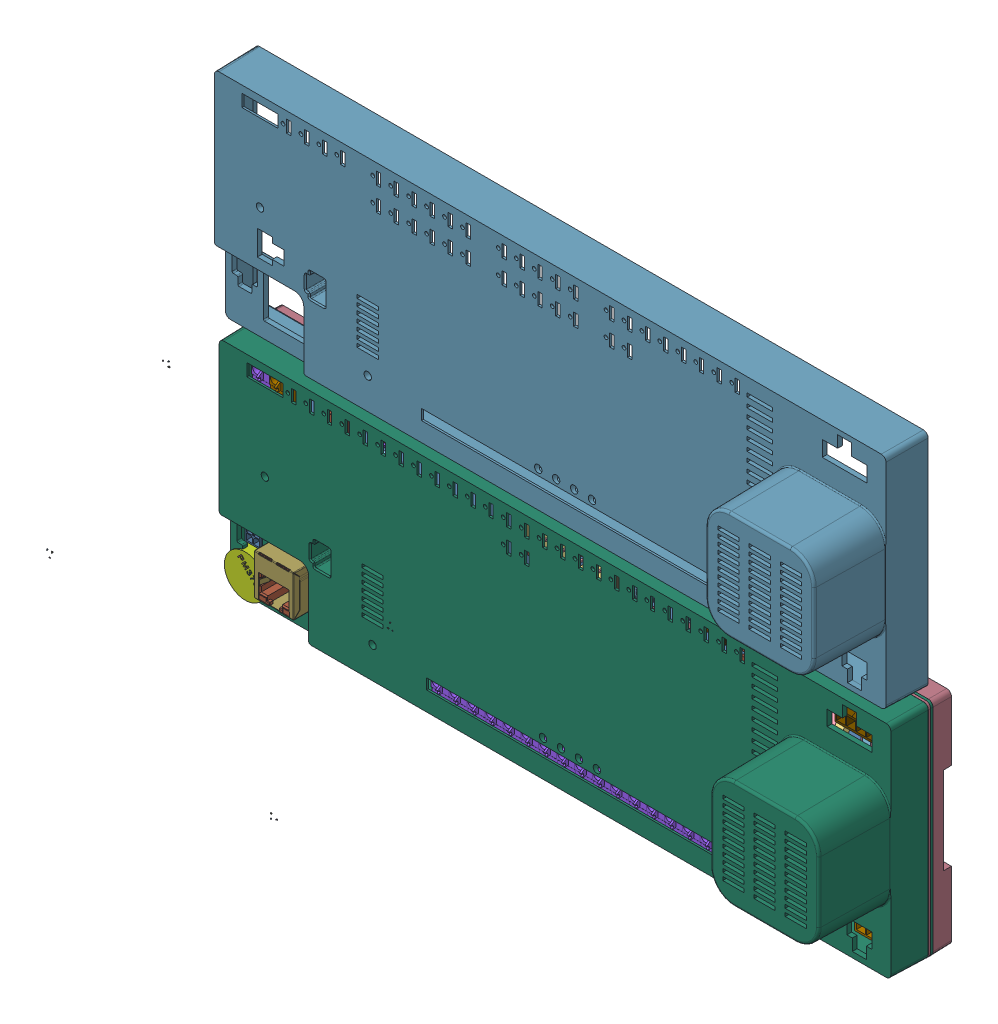
SolidWorks assembly _SC944D, configuration Default. Lengths in mm. (continued)
Components (placement in the parent): (continued)
- U10-1: U10 [Default] at origin size (22 22 1.6) (continued)
  - User_Library-LQFP144-1: User_Library-LQFP144 [Default] at (60.232 23.8429 0) x (-1 0 0) z (0 1 0) size (22 1.6 22) (continued)
    - User_Library-LQFP144_Assu_Fuss_LQFP144-2: User_Library-LQFP144_Assu_Fuss_LQFP144 [Default] at (0 0 -10) x (0 0 -1) z (1 0 0) size (1 0.89 17.72) (continued)
      - User_Library-LQFP144_Fuss_LQFP144-319: User_Library-LQFP144_Fuss_LQFP144 [Default] at (0 0 4.25) size (1 0.89 0.22)
      - User_Library-LQFP144_Fuss_LQFP144-320: User_Library-LQFP144_Fuss_LQFP144 [Default] at (0 0 -1.25) size (1 0.89 0.22)
      - User_Library-LQFP144_Fuss_LQFP144-321: User_Library-LQFP144_Fuss_LQFP144 [Default] at (0 0 -3.75) size (1 0.89 0.22)
      - User_Library-LQFP144_Fuss_LQFP144-322: User_Library-LQFP144_Fuss_LQFP144 [Default] at (0 0 -2.25) size (1 0.89 0.22)
      - User_Library-LQFP144_Fuss_LQFP144-323: User_Library-LQFP144_Fuss_LQFP144 [Default] at (0 0 3.25) size (1 0.89 0.22)
      - User_Library-LQFP144_Fuss_LQFP144-324: User_Library-LQFP144_Fuss_LQFP144 [Default] at (0 0 1.25) size (1 0.89 0.22)
      - User_Library-LQFP144_Fuss_LQFP144-325: User_Library-LQFP144_Fuss_LQFP144 [Default] at (0 0 0.25) size (1 0.89 0.22)
      - User_Library-LQFP144_Fuss_LQFP144-326: User_Library-LQFP144_Fuss_LQFP144 [Default] at (0 0 2.75) size (1 0.89 0.22)
      - User_Library-LQFP144_Fuss_LQFP144-327: User_Library-LQFP144_Fuss_LQFP144 [Default] at (0 0 -2.75) size (1 0.89 0.22)
      - User_Library-LQFP144_Fuss_LQFP144-328: User_Library-LQFP144_Fuss_LQFP144 [Default] at (0 0 -3.75) size (1 0.89 0.22)
      - User_Library-LQFP144_Fuss_LQFP144-329: User_Library-LQFP144_Fuss_LQFP144 [Default] at (0 0 -0.25) size (1 0.89 0.22)
      - User_Library-LQFP144_Fuss_LQFP144-330: User_Library-LQFP144_Fuss_LQFP144 [Default] at (0 0 -2.75) size (1 0.89 0.22)
      - User_Library-LQFP144_Fuss_LQFP144-331: User_Library-LQFP144_Fuss_LQFP144 [Default] at (0 0 -5.25) size (1 0.89 0.22)
      - User_Library-LQFP144_Fuss_LQFP144-332: User_Library-LQFP144_Fuss_LQFP144 [Default] at (0 0 -2.25) size (1 0.89 0.22)
      - User_Library-LQFP144_Fuss_LQFP144-333: User_Library-LQFP144_Fuss_LQFP144 [Default] at (0 0 0.75) size (1 0.89 0.22)
      - User_Library-LQFP144_Fuss_LQFP144-334: User_Library-LQFP144_Fuss_LQFP144 [Default] at (0 0 5.25) size (1 0.89 0.22)
      - User_Library-LQFP144_Fuss_LQFP144-335: User_Library-LQFP144_Fuss_LQFP144 [Default] at (0 0 -1.25) size (1 0.89 0.22)
      - User_Library-LQFP144_Fuss_LQFP144-336: User_Library-LQFP144_Fuss_LQFP144 [Default] at (0 0 2.25) size (1 0.89 0.22)
      - User_Library-LQFP144_Fuss_LQFP144-337: User_Library-LQFP144_Fuss_LQFP144 [Default] at (0 0 3.75) size (1 0.89 0.22)
      - User_Library-LQFP144_Fuss_LQFP144-338: User_Library-LQFP144_Fuss_LQFP144 [Default] at (0 0 2.25) size (1 0.89 0.22)
      - User_Library-LQFP144_Fuss_LQFP144-339: User_Library-LQFP144_Fuss_LQFP144 [Default] at (0 0 4.75) size (1 0.89 0.22)
      - User_Library-LQFP144_Fuss_LQFP144-340: User_Library-LQFP144_Fuss_LQFP144 [Default] at (0 0 0.75) size (1 0.89 0.22)
      - User_Library-LQFP144_Fuss_LQFP144-341: User_Library-LQFP144_Fuss_LQFP144 [Default] at (0 0 3.25) size (1 0.89 0.22)
      - User_Library-LQFP144_Fuss_LQFP144-342: User_Library-LQFP144_Fuss_LQFP144 [Default] at (0 0 2.75) size (1 0.89 0.22)
    - User_Library-LQFP144_Assu_Fuss_LQFP144-3: User_Library-LQFP144_Assu_Fuss_LQFP144 [Default] at (0 0 10) x (0 0 1) z (-1 0 0) size (1 0.89 17.72)
      - User_Library-LQFP144_Fuss_LQFP144-1: User_Library-LQFP144_Fuss_LQFP144 [Default] at (0 0 3.25) size (1 0.89 0.22)
      - User_Library-LQFP144_Fuss_LQFP144-2: User_Library-LQFP144_Fuss_LQFP144 [Default] at (0 0 -5.75) size (1 0.89 0.22)
      - User_Library-LQFP144_Fuss_LQFP144-3: User_Library-LQFP144_Fuss_LQFP144 [Default] at (0 0 -3.75) size (1 0.89 0.22)
      - User_Library-LQFP144_Fuss_LQFP144-4: User_Library-LQFP144_Fuss_LQFP144 [Default] at (0 0 -0.25) size (1 0.89 0.22)
      - User_Library-LQFP144_Fuss_LQFP144-5: User_Library-LQFP144_Fuss_LQFP144 [Default] at (0 0 -5.25) size (1 0.89 0.22)
      - User_Library-LQFP144_Fuss_LQFP144-6: User_Library-LQFP144_Fuss_LQFP144 [Default] at (0 0 -8.25) size (1 0.89 0.22)
      - User_Library-LQFP144_Fuss_LQFP144-7: User_Library-LQFP144_Fuss_LQFP144 [Default] at (0 0 -0.25) size (1 0.89 0.22)
      - User_Library-LQFP144_Fuss_LQFP144-8: User_Library-LQFP144_Fuss_LQFP144 [Default] at (0 0 -3.75) size (1 0.89 0.22)
      - User_Library-LQFP144_Fuss_LQFP144-9: User_Library-LQFP144_Fuss_LQFP144 [Default] at (0 0 -0.25) size (1 0.89 0.22)
      - User_Library-LQFP144_Fuss_LQFP144-10: User_Library-LQFP144_Fuss_LQFP144 [Default] at (0 0 6.75) size (1 0.89 0.22)
      - User_Library-LQFP144_Fuss_LQFP144-11: User_Library-LQFP144_Fuss_LQFP144 [Default] at (0 0 -3.75) size (1 0.89 0.22)
      - User_Library-LQFP144_Fuss_LQFP144-12: User_Library-LQFP144_Fuss_LQFP144 [Default] at (0 0 4.25) size (1 0.89 0.22)
      - User_Library-LQFP144_Fuss_LQFP144-13: User_Library-LQFP144_Fuss_LQFP144 [Default] at (0 0 0.75) size (1 0.89 0.22)
      - User_Library-LQFP144_Fuss_LQFP144-14: User_Library-LQFP144_Fuss_LQFP144 [Default] at (0 0 7.75) size (1 0.89 0.22)
      - User_Library-LQFP144_Fuss_LQFP144-15: User_Library-LQFP144_Fuss_LQFP144 [Default] at (0 0 1.75) size (1 0.89 0.22)
      - User_Library-LQFP144_Fuss_LQFP144-16: User_Library-LQFP144_Fuss_LQFP144 [Default] at (0 0 -2.25) size (1 0.89 0.22)
      - User_Library-LQFP144_Fuss_LQFP144-17: User_Library-LQFP144_Fuss_LQFP144 [Default] at (0 0 -2.75) size (1 0.89 0.22)
      - User_Library-LQFP144_Fuss_LQFP144-18: User_Library-LQFP144_Fuss_LQFP144 [Default] at (0 0 -4.25) size (1 0.89 0.22)
      - User_Library-LQFP144_Fuss_LQFP144-19: User_Library-LQFP144_Fuss_LQFP144 [Default] at (0 0 3.25) size (1 0.89 0.22)
      - User_Library-LQFP144_Fuss_LQFP144-20: User_Library-LQFP144_Fuss_LQFP144 [Default] at (0 0 -1.75) size (1 0.89 0.22)
      - User_Library-LQFP144_Fuss_LQFP144-21: User_Library-LQFP144_Fuss_LQFP144 [Default] at (0 0 -1.75) size (1 0.89 0.22)
      - User_Library-LQFP144_Fuss_LQFP144-22: User_Library-LQFP144_Fuss_LQFP144 [Default] at (0 0 2.75) size (1 0.89 0.22)
      - User_Library-LQFP144_Fuss_LQFP144-23: User_Library-LQFP144_Fuss_LQFP144 [Default] at (0 0 -2.75) size (1 0.89 0.22)
      - User_Library-LQFP144_Fuss_LQFP144-24: User_Library-LQFP144_Fuss_LQFP144 [Default] at (0 0 -3.75) size (1 0.89 0.22)
      - User_Library-LQFP144_Fuss_LQFP144-25: User_Library-LQFP144_Fuss_LQFP144 [Default] at (0 0 -5.75) size (1 0.89 0.22)
      - User_Library-LQFP144_Fuss_LQFP144-26: User_Library-LQFP144_Fuss_LQFP144 [Default] at (0 0 0.75) size (1 0.89 0.22)
      - User_Library-LQFP144_Fuss_LQFP144-27: User_Library-LQFP144_Fuss_LQFP144 [Default] at (0 0 -6.25) size (1 0.89 0.22)
      - User_Library-LQFP144_Fuss_LQFP144-28: User_Library-LQFP144_Fuss_LQFP144 [Default] at (0 0 -2.75) size (1 0.89 0.22)
      - User_Library-LQFP144_Fuss_LQFP144-29: User_Library-LQFP144_Fuss_LQFP144 [Default] at (0 0 1.25) size (1 0.89 0.22)
      - User_Library-LQFP144_Fuss_LQFP144-30: User_Library-LQFP144_Fuss_LQFP144 [Default] at (0 0 -0.25) size (1 0.89 0.22)
      - User_Library-LQFP144_Fuss_LQFP144-31: User_Library-LQFP144_Fuss_LQFP144 [Default] at (0 0 -1.25) size (1 0.89 0.22)
      - User_Library-LQFP144_Fuss_LQFP144-32: User_Library-LQFP144_Fuss_LQFP144 [Default] at (0 0 5.25) size (1 0.89 0.22)
      - User_Library-LQFP144_Fuss_LQFP144-33: User_Library-LQFP144_Fuss_LQFP144 [Default] at (0 0 8.25) size (1 0.89 0.22)
      - User_Library-LQFP144_Fuss_LQFP144-34: User_Library-LQFP144_Fuss_LQFP144 [Default] at (0 0 -6.25) size (1 0.89 0.22)
      - User_Library-LQFP144_Fuss_LQFP144-35: User_Library-LQFP144_Fuss_LQFP144 [Default] at (0 0 -0.75) size (1 0.89 0.22)
      - User_Library-LQFP144_Fuss_LQFP144-36: User_Library-LQFP144_Fuss_LQFP144 [Default] at (0 0 -8.75) size (1 0.89 0.22)
      - User_Library-LQFP144_Fuss_LQFP144-37: User_Library-LQFP144_Fuss_LQFP144 [Default] at (0 0 -1.25) size (1 0.89 0.22)
      - User_Library-LQFP144_Fuss_LQFP144-38: User_Library-LQFP144_Fuss_LQFP144 [Default] at (0 0 -1.25) size (1 0.89 0.22)
      - User_Library-LQFP144_Fuss_LQFP144-39: User_Library-LQFP144_Fuss_LQFP144 [Default] at (0 0 -2.75) size (1 0.89 0.22)
      - User_Library-LQFP144_Fuss_LQFP144-40: User_Library-LQFP144_Fuss_LQFP144 [Default] at (0 0 -2.75) size (1 0.89 0.22)
      - User_Library-LQFP144_Fuss_LQFP144-41: User_Library-LQFP144_Fuss_LQFP144 [Default] at (0 0 2.25) size (1 0.89 0.22)
      - User_Library-LQFP144_Fuss_LQFP144-42: User_Library-LQFP144_Fuss_LQFP144 [Default] at (0 0 3.75) size (1 0.89 0.22)
      - User_Library-LQFP144_Fuss_LQFP144-43: User_Library-LQFP144_Fuss_LQFP144 [Default] at (0 0 0.75) size (1 0.89 0.22)
      - User_Library-LQFP144_Fuss_LQFP144-44: User_Library-LQFP144_Fuss_LQFP144 [Default] at (0 0 0.75) size (1 0.89 0.22)
      - User_Library-LQFP144_Fuss_LQFP144-45: User_Library-LQFP144_Fuss_LQFP144 [Default] at (0 0 1.25) size (1 0.89 0.22)
      - User_Library-LQFP144_Fuss_LQFP144-46: User_Library-LQFP144_Fuss_LQFP144 [Default] at (0 0 1.75) size (1 0.89 0.22)
      - User_Library-LQFP144_Fuss_LQFP144-47: User_Library-LQFP144_Fuss_LQFP144 [Default] at (0 0 3.25) size (1 0.89 0.22)
      - User_Library-LQFP144_Fuss_LQFP144-48: User_Library-LQFP144_Fuss_LQFP144 [Default] at (0 0 -3.25) size (1 0.89 0.22)
      - User_Library-LQFP144_Fuss_LQFP144-49: User_Library-LQFP144_Fuss_LQFP144 [Default] at (0 0 5.75) size (1 0.89 0.22)
      - User_Library-LQFP144_Fuss_LQFP144-50: User_Library-LQFP144_Fuss_LQFP144 [Default] at (0 0 4.25) size (1 0.89 0.22)
      - User_Library-LQFP144_Fuss_LQFP144-51: User_Library-LQFP144_Fuss_LQFP144 [Default] at (0 0 3.25) size (1 0.89 0.22)
      - User_Library-LQFP144_Fuss_LQFP144-52: User_Library-LQFP144_Fuss_LQFP144 [Default] at (0 0 6.25) size (1 0.89 0.22)
      - User_Library-LQFP144_Fuss_LQFP144-53: User_Library-LQFP144_Fuss_LQFP144 [Default] at (0 0 -5.25) size (1 0.89 0.22)
      - User_Library-LQFP144_Fuss_LQFP144-54: User_Library-LQFP144_Fuss_LQFP144 [Default] at (0 0 -6.75) size (1 0.89 0.22)
      - User_Library-LQFP144_Fuss_LQFP144-55: User_Library-LQFP144_Fuss_LQFP144 [Default] at (0 0 -0.75) size (1 0.89 0.22)
      - User_Library-LQFP144_Fuss_LQFP144-56: User_Library-LQFP144_Fuss_LQFP144 [Default] at (0 0 1.75) size (1 0.89 0.22)
      - User_Library-LQFP144_Fuss_LQFP144-57: User_Library-LQFP144_Fuss_LQFP144 [Default] at (0 0 -3.25) size (1 0.89 0.22)
      - User_Library-LQFP144_Fuss_LQFP144-58: User_Library-LQFP144_Fuss_LQFP144 [Default] at (0 0 -4.25) size (1 0.89 0.22)
      - User_Library-LQFP144_Fuss_LQFP144-59: User_Library-LQFP144_Fuss_LQFP144 [Default] at (0 0 -5.25) size (1 0.89 0.22)
      - User_Library-LQFP144_Fuss_LQFP144-60: User_Library-LQFP144_Fuss_LQFP144 [Default] at (0 0 -1.25) size (1 0.89 0.22)
      - User_Library-LQFP144_Fuss_LQFP144-61: User_Library-LQFP144_Fuss_LQFP144 [Default] at (0 0 -0.75) size (1 0.89 0.22)
      - User_Library-LQFP144_Fuss_LQFP144-62: User_Library-LQFP144_Fuss_LQFP144 [Default] at (0 0 -6.25) size (1 0.89 0.22)
      - User_Library-LQFP144_Fuss_LQFP144-63: User_Library-LQFP144_Fuss_LQFP144 [Default] at (0 0 4.75) size (1 0.89 0.22)
      - User_Library-LQFP144_Fuss_LQFP144-64: User_Library-LQFP144_Fuss_LQFP144 [Default] at (0 0 3.25) size (1 0.89 0.22)
      - User_Library-LQFP144_Fuss_LQFP144-65: User_Library-LQFP144_Fuss_LQFP144 [Default] at (0 0 4.25) size (1 0.89 0.22)
      - User_Library-LQFP144_Fuss_LQFP144-66: User_Library-LQFP144_Fuss_LQFP144 [Default] at (0 0 0.25) size (1 0.89 0.22)
      - User_Library-LQFP144_Fuss_LQFP144-67: User_Library-LQFP144_Fuss_LQFP144 [Default] at (0 0 4.25) size (1 0.89 0.22)
      - User_Library-LQFP144_Fuss_LQFP144-68: User_Library-LQFP144_Fuss_LQFP144 [Default] at (0 0 6.75) size (1 0.89 0.22)
      - User_Library-LQFP144_Fuss_LQFP144-69: User_Library-LQFP144_Fuss_LQFP144 [Default] at (0 0 0.25) size (1 0.89 0.22)
      - User_Library-LQFP144_Fuss_LQFP144-70: User_Library-LQFP144_Fuss_LQFP144 [Default] at (0 0 0.25) size (1 0.89 0.22)
      - User_Library-LQFP144_Fuss_LQFP144-71: User_Library-LQFP144_Fuss_LQFP144 [Default] at (0 0 -1.25) size (1 0.89 0.22)
      - User_Library-LQFP144_Fuss_LQFP144-72: User_Library-LQFP144_Fuss_LQFP144 [Default] at (0 0 -3.75) size (1 0.89 0.22)
      - User_Library-LQFP144_Fuss_LQFP144-73: User_Library-LQFP144_Fuss_LQFP144 [Default] at (0 0 -0.25) size (1 0.89 0.22)
      - User_Library-LQFP144_Fuss_LQFP144-74: User_Library-LQFP144_Fuss_LQFP144 [Default] at (0 0 1.25) size (1 0.89 0.22)
      - User_Library-LQFP144_Fuss_LQFP144-75: User_Library-LQFP144_Fuss_LQFP144 [Default] at (0 0 0.75) size (1 0.89 0.22)
      - User_Library-LQFP144_Fuss_LQFP144-76: User_Library-LQFP144_Fuss_LQFP144 [Default] at (0 0 -7.75) size (1 0.89 0.22)
      - User_Library-LQFP144_Fuss_LQFP144-77: User_Library-LQFP144_Fuss_LQFP144 [Default] at (0 0 -3.25) size (1 0.89 0.22)
      - User_Library-LQFP144_Fuss_LQFP144-78: User_Library-LQFP144_Fuss_LQFP144 [Default] at (0 0 2.75) size (1 0.89 0.22)
      - User_Library-LQFP144_Fuss_LQFP144-79: User_Library-LQFP144_Fuss_LQFP144 [Default] at (0 0 4.75) size (1 0.89 0.22)
      - User_Library-LQFP144_Fuss_LQFP144-80: User_Library-LQFP144_Fuss_LQFP144 [Default] at (0 0 -7.25) size (1 0.89 0.22)
      - User_Library-LQFP144_Fuss_LQFP144-81: User_Library-LQFP144_Fuss_LQFP144 [Default] at (0 0 0.75) size (1 0.89 0.22)
      - User_Library-LQFP144_Fuss_LQFP144-82: User_Library-LQFP144_Fuss_LQFP144 [Default] at (0 0 0.75) size (1 0.89 0.22)
      - User_Library-LQFP144_Fuss_LQFP144-83: User_Library-LQFP144_Fuss_LQFP144 [Default] at (0 0 -0.75) size (1 0.89 0.22)
      - User_Library-LQFP144_Fuss_LQFP144-84: User_Library-LQFP144_Fuss_LQFP144 [Default] at (0 0 6.75) size (1 0.89 0.22)
      - User_Library-LQFP144_Fuss_LQFP144-85: User_Library-LQFP144_Fuss_LQFP144 [Default] at (0 0 -3.25) size (1 0.89 0.22)
      - User_Library-LQFP144_Fuss_LQFP144-86: User_Library-LQFP144_Fuss_LQFP144 [Default] at (0 0 3.75) size (1 0.89 0.22)
      - User_Library-LQFP144_Fuss_LQFP144-87: User_Library-LQFP144_Fuss_LQFP144 [Default] at (0 0 -0.75) size (1 0.89 0.22)
      - User_Library-LQFP144_Fuss_LQFP144-88: User_Library-LQFP144_Fuss_LQFP144 [Default] at (0 0 -1.75) size (1 0.89 0.22)
      - User_Library-LQFP144_Fuss_LQFP144-89: User_Library-LQFP144_Fuss_LQFP144 [Default] at (0 0 7.25) size (1 0.89 0.22)
      - User_Library-LQFP144_Fuss_LQFP144-90: User_Library-LQFP144_Fuss_LQFP144 [Default] at (0 0 0.75) size (1 0.89 0.22)
      - User_Library-LQFP144_Fuss_LQFP144-91: User_Library-LQFP144_Fuss_LQFP144 [Default] at (0 0 0.25) size (1 0.89 0.22)
      - User_Library-LQFP144_Fuss_LQFP144-92: User_Library-LQFP144_Fuss_LQFP144 [Default] at (0 0 0.25) size (1 0.89 0.22)
      - User_Library-LQFP144_Fuss_LQFP144-93: User_Library-LQFP144_Fuss_LQFP144 [Default] at (0 0 0.25) size (1 0.89 0.22)
      - User_Library-LQFP144_Fuss_LQFP144-94: User_Library-LQFP144_Fuss_LQFP144 [Default] at (0 0 1.75) size (1 0.89 0.22)
      - User_Library-LQFP144_Fuss_LQFP144-95: User_Library-LQFP144_Fuss_LQFP144 [Default] at (0 0 3.25) size (1 0.89 0.22)
      - User_Library-LQFP144_Fuss_LQFP144-96: User_Library-LQFP144_Fuss_LQFP144 [Default] at (0 0 -2.75) size (1 0.89 0.22)
      - User_Library-LQFP144_Fuss_LQFP144-97: User_Library-LQFP144_Fuss_LQFP144 [Default] at (0 0 -1.75) size (1 0.89 0.22)
      - User_Library-LQFP144_Fuss_LQFP144-98: User_Library-LQFP144_Fuss_LQFP144 [Default] at (0 0 4.75) size (1 0.89 0.22)
      - User_Library-LQFP144_Fuss_LQFP144-99: User_Library-LQFP144_Fuss_LQFP144 [Default] at (0 0 1.25) size (1 0.89 0.22)
      - User_Library-LQFP144_Fuss_LQFP144-100: User_Library-LQFP144_Fuss_LQFP144 [Default] at (0 0 4.75) size (1 0.89 0.22)
      - User_Library-LQFP144_Fuss_LQFP144-101: User_Library-LQFP144_Fuss_LQFP144 [Default] at (0 0 2.25) size (1 0.89 0.22)
      - User_Library-LQFP144_Fuss_LQFP144-102: User_Library-LQFP144_Fuss_LQFP144 [Default] at (0 0 2.25) size (1 0.89 0.22)
      - User_Library-LQFP144_Fuss_LQFP144-103: User_Library-LQFP144_Fuss_LQFP144 [Default] at (0 0 -2.75) size (1 0.89 0.22)
      - User_Library-LQFP144_Fuss_LQFP144-104: User_Library-LQFP144_Fuss_LQFP144 [Default] at (0 0 1.75) size (1 0.89 0.22)
      - User_Library-LQFP144_Fuss_LQFP144-105: User_Library-LQFP144_Fuss_LQFP144 [Default] at (0 0 7.25) size (1 0.89 0.22)
      - User_Library-LQFP144_Fuss_LQFP144-106: User_Library-LQFP144_Fuss_LQFP144 [Default] at (0 0 4.25) size (1 0.89 0.22)
      - User_Library-LQFP144_Fuss_LQFP144-107: User_Library-LQFP144_Fuss_LQFP144 [Default] at (0 0 7.75) size (1 0.89 0.22)
      - User_Library-LQFP144_Fuss_LQFP144-108: User_Library-LQFP144_Fuss_LQFP144 [Default] at (0 0 4.25) size (1 0.89 0.22)
      - User_Library-LQFP144_Fuss_LQFP144-109: User_Library-LQFP144_Fuss_LQFP144 [Default] at (0 0 7.25) size (1 0.89 0.22)
      - User_Library-LQFP144_Fuss_LQFP144-110: User_Library-LQFP144_Fuss_LQFP144 [Default] at (0 0 1.25) size (1 0.89 0.22)
      - User_Library-LQFP144_Fuss_LQFP144-111: User_Library-LQFP144_Fuss_LQFP144 [Default] at (0 0 7.25) size (1 0.89 0.22)
      - User_Library-LQFP144_Fuss_LQFP144-112: User_Library-LQFP144_Fuss_LQFP144 [Default] at (0 0 5.25) size (1 0.89 0.22)
      - User_Library-LQFP144_Fuss_LQFP144-113: User_Library-LQFP144_Fuss_LQFP144 [Default] at (0 0 6.75) size (1 0.89 0.22)
      - User_Library-LQFP144_Fuss_LQFP144-114: User_Library-LQFP144_Fuss_LQFP144 [Default] at (0 0 -6.25) size (1 0.89 0.22)
      - User_Library-LQFP144_Fuss_LQFP144-115: User_Library-LQFP144_Fuss_LQFP144 [Default] at (0 0 -0.25) size (1 0.89 0.22)
      - User_Library-LQFP144_Fuss_LQFP144-116: User_Library-LQFP144_Fuss_LQFP144 [Default] at (0 0 0.25) size (1 0.89 0.22)
      - User_Library-LQFP144_Fuss_LQFP144-117: User_Library-LQFP144_Fuss_LQFP144 [Default] at (0 0 8.25) size (1 0.89 0.22)
      - User_Library-LQFP144_Fuss_LQFP144-118: User_Library-LQFP144_Fuss_LQFP144 [Default] at (0 0 -4.75) size (1 0.89 0.22)
      - User_Library-LQFP144_Fuss_LQFP144-119: User_Library-LQFP144_Fuss_LQFP144 [Default] at (0 0 -2.25) size (1 0.89 0.22)
      - User_Library-LQFP144_Fuss_LQFP144-120: User_Library-LQFP144_Fuss_LQFP144 [Default] at (0 0 -6.75) size (1 0.89 0.22)
      - User_Library-LQFP144_Fuss_LQFP144-121: User_Library-LQFP144_Fuss_LQFP144 [Default] at (0 0 -1.75) size (1 0.89 0.22)
      - User_Library-LQFP144_Fuss_LQFP144-122: User_Library-LQFP144_Fuss_LQFP144 [Default] at (0 0 -7.25) size (1 0.89 0.22)
      - User_Library-LQFP144_Fuss_LQFP144-123: User_Library-LQFP144_Fuss_LQFP144 [Default] at (0 0 -5.25) size (1 0.89 0.22)
      - User_Library-LQFP144_Fuss_LQFP144-124: User_Library-LQFP144_Fuss_LQFP144 [Default] at (0 0 -5.75) size (1 0.89 0.22)
      - User_Library-LQFP144_Fuss_LQFP144-125: User_Library-LQFP144_Fuss_LQFP144 [Default] at (0 0 2.75) size (1 0.89 0.22)
      - User_Library-LQFP144_Fuss_LQFP144-126: User_Library-LQFP144_Fuss_LQFP144 [Default] at (0 0 1.75) size (1 0.89 0.22)
      - User_Library-LQFP144_Fuss_LQFP144-127: User_Library-LQFP144_Fuss_LQFP144 [Default] at (0 0 0.25) size (1 0.89 0.22)
      - User_Library-LQFP144_Fuss_LQFP144-128: User_Library-LQFP144_Fuss_LQFP144 [Default] at (0 0 -3.25) size (1 0.89 0.22)
      - User_Library-LQFP144_Fuss_LQFP144-129: User_Library-LQFP144_Fuss_LQFP144 [Default] at (0 0 3.25) size (1 0.89 0.22)
      - User_Library-LQFP144_Fuss_LQFP144-130: User_Library-LQFP144_Fuss_LQFP144 [Default] at (0 0 -2.75) size (1 0.89 0.22)
      - User_Library-LQFP144_Fuss_LQFP144-131: User_Library-LQFP144_Fuss_LQFP144 [Default] at (0 0 3.75) size (1 0.89 0.22)
      - User_Library-LQFP144_Fuss_LQFP144-132: User_Library-LQFP144_Fuss_LQFP144 [Default] at (0 0 0.25) size (1 0.89 0.22)
      - User_Library-LQFP144_Fuss_LQFP144-133: User_Library-LQFP144_Fuss_LQFP144 [Default] at (0 0 2.25) size (1 0.89 0.22)
      - User_Library-LQFP144_Fuss_LQFP144-134: User_Library-LQFP144_Fuss_LQFP144 [Default] at (0 0 -1.25) size (1 0.89 0.22)
      - User_Library-LQFP144_Fuss_LQFP144-135: User_Library-LQFP144_Fuss_LQFP144 [Default] at (0 0 -0.75) size (1 0.89 0.22)
      - User_Library-LQFP144_Fuss_LQFP144-136: User_Library-LQFP144_Fuss_LQFP144 [Default] at (0 0 -4.25) size (1 0.89 0.22)
      - User_Library-LQFP144_Fuss_LQFP144-137: User_Library-LQFP144_Fuss_LQFP144 [Default] at (0 0 1.75) size (1 0.89 0.22)
      - User_Library-LQFP144_Fuss_LQFP144-138: User_Library-LQFP144_Fuss_LQFP144 [Default] at (0 0 -1.25) size (1 0.89 0.22)
      - User_Library-LQFP144_Fuss_LQFP144-139: User_Library-LQFP144_Fuss_LQFP144 [Default] at (0 0 -1.75) size (1 0.89 0.22)
      - User_Library-LQFP144_Fuss_LQFP144-140: User_Library-LQFP144_Fuss_LQFP144 [Default] at (0 0 4.25) size (1 0.89 0.22)
      - User_Library-LQFP144_Fuss_LQFP144-141: User_Library-LQFP144_Fuss_LQFP144 [Default] at (0 0 -2.25) size (1 0.89 0.22)
      - User_Library-LQFP144_Fuss_LQFP144-142: User_Library-LQFP144_Fuss_LQFP144 [Default] at (0 0 5.25) size (1 0.89 0.22)
      - User_Library-LQFP144_Fuss_LQFP144-143: User_Library-LQFP144_Fuss_LQFP144 [Default] at (0 0 2.75) size (1 0.89 0.22)
      - User_Library-LQFP144_Fuss_LQFP144-144: User_Library-LQFP144_Fuss_LQFP144 [Default] at (0 0 -1.75) size (1 0.89 0.22)
      - User_Library-LQFP144_Fuss_LQFP144-145: User_Library-LQFP144_Fuss_LQFP144 [Default] at (0 0 -0.25) size (1 0.89 0.22)
      - User_Library-LQFP144_Fuss_LQFP144-146: User_Library-LQFP144_Fuss_LQFP144 [Default] at (0 0 0.75) size (1 0.89 0.22)
      - User_Library-LQFP144_Fuss_LQFP144-147: User_Library-LQFP144_Fuss_LQFP144 [Default] at (0 0 -0.25) size (1 0.89 0.22)
      - User_Library-LQFP144_Fuss_LQFP144-148: User_Library-LQFP144_Fuss_LQFP144 [Default] at (0 0 3.75) size (1 0.89 0.22)
      - User_Library-LQFP144_Fuss_LQFP144-149: User_Library-LQFP144_Fuss_LQFP144 [Default] at (0 0 2.75) size (1 0.89 0.22)
      - User_Library-LQFP144_Fuss_LQFP144-150: User_Library-LQFP144_Fuss_LQFP144 [Default] at (0 0 2.75) size (1 0.89 0.22)
      - User_Library-LQFP144_Fuss_LQFP144-151: User_Library-LQFP144_Fuss_LQFP144 [Default] at (0 0 6.25) size (1 0.89 0.22)
      - User_Library-LQFP144_Fuss_LQFP144-152: User_Library-LQFP144_Fuss_LQFP144 [Default] at (0 0 2.25) size (1 0.89 0.22)
      - User_Library-LQFP144_Fuss_LQFP144-153: User_Library-LQFP144_Fuss_LQFP144 [Default] at (0 0 -0.75) size (1 0.89 0.22)
      - User_Library-LQFP144_Fuss_LQFP144-154: User_Library-LQFP144_Fuss_LQFP144 [Default] at (0 0 -2.25) size (1 0.89 0.22)
      - User_Library-LQFP144_Fuss_LQFP144-155: User_Library-LQFP144_Fuss_LQFP144 [Default] at (0 0 -0.75) size (1 0.89 0.22)
      - User_Library-LQFP144_Fuss_LQFP144-156: User_Library-LQFP144_Fuss_LQFP144 [Default] at (0 0 -2.25) size (1 0.89 0.22)
      - User_Library-LQFP144_Fuss_LQFP144-157: User_Library-LQFP144_Fuss_LQFP144 [Default] at (0 0 -2.25) size (1 0.89 0.22)
      - User_Library-LQFP144_Fuss_LQFP144-158: User_Library-LQFP144_Fuss_LQFP144 [Default] at (0 0 0.75) size (1 0.89 0.22)
      - User_Library-LQFP144_Fuss_LQFP144-159: User_Library-LQFP144_Fuss_LQFP144 [Default] at (0 0 -4.25) size (1 0.89 0.22)
      - User_Library-LQFP144_Fuss_LQFP144-160: User_Library-LQFP144_Fuss_LQFP144 [Default] at (0 0 4.25) size (1 0.89 0.22)
      - User_Library-LQFP144_Fuss_LQFP144-161: User_Library-LQFP144_Fuss_LQFP144 [Default] at (0 0 1.25) size (1 0.89 0.22)
      - User_Library-LQFP144_Fuss_LQFP144-162: User_Library-LQFP144_Fuss_LQFP144 [Default] at (0 0 -0.25) size (1 0.89 0.22)
      - User_Library-LQFP144_Fuss_LQFP144-163: User_Library-LQFP144_Fuss_LQFP144 [Default] at (0 0 -4.25) size (1 0.89 0.22)
      - User_Library-LQFP144_Fuss_LQFP144-164: User_Library-LQFP144_Fuss_LQFP144 [Default] at (0 0 -1.25) size (1 0.89 0.22)
      - User_Library-LQFP144_Fuss_LQFP144-165: User_Library-LQFP144_Fuss_LQFP144 [Default] at (0 0 -8.25) size (1 0.89 0.22)
      - User_Library-LQFP144_Fuss_LQFP144-166: User_Library-LQFP144_Fuss_LQFP144 [Default] at (0 0 -3.25) size (1 0.89 0.22)
      - User_Library-LQFP144_Fuss_LQFP144-167: User_Library-LQFP144_Fuss_LQFP144 [Default] at (0 0 -4.75) size (1 0.89 0.22)
      - User_Library-LQFP144_Fuss_LQFP144-168: User_Library-LQFP144_Fuss_LQFP144 [Default] at (0 0 -2.25) size (1 0.89 0.22)
      - User_Library-LQFP144_Fuss_LQFP144-169: User_Library-LQFP144_Fuss_LQFP144 [Default] at (0 0 -1.25) size (1 0.89 0.22)
      - User_Library-LQFP144_Fuss_LQFP144-170: User_Library-LQFP144_Fuss_LQFP144 [Default] at (0 0 -7.25) size (1 0.89 0.22)
      - User_Library-LQFP144_Fuss_LQFP144-171: User_Library-LQFP144_Fuss_LQFP144 [Default] at (0 0 -4.25) size (1 0.89 0.22)
      - User_Library-LQFP144_Fuss_LQFP144-172: User_Library-LQFP144_Fuss_LQFP144 [Default] at (0 0 -4.25) size (1 0.89 0.22)
      - User_Library-LQFP144_Fuss_LQFP144-173: User_Library-LQFP144_Fuss_LQFP144 [Default] at (0 0 1.75) size (1 0.89 0.22)
      - User_Library-LQFP144_Fuss_LQFP144-174: User_Library-LQFP144_Fuss_LQFP144 [Default] at (0 0 0.25) size (1 0.89 0.22)
      - User_Library-LQFP144_Fuss_LQFP144-175: User_Library-LQFP144_Fuss_LQFP144 [Default] at (0 0 -0.75) size (1 0.89 0.22)
      - User_Library-LQFP144_Fuss_LQFP144-176: User_Library-LQFP144_Fuss_LQFP144 [Default] at (0 0 0.75) size (1 0.89 0.22)
      - User_Library-LQFP144_Fuss_LQFP144-177: User_Library-LQFP144_Fuss_LQFP144 [Default] at (0 0 1.75) size (1 0.89 0.22)
      - User_Library-LQFP144_Fuss_LQFP144-178: User_Library-LQFP144_Fuss_LQFP144 [Default] at (0 0 -0.75) size (1 0.89 0.22)
      - User_Library-LQFP144_Fuss_LQFP144-179: User_Library-LQFP144_Fuss_LQFP144 [Default] at (0 0 3.75) size (1 0.89 0.22)
      - User_Library-LQFP144_Fuss_LQFP144-180: User_Library-LQFP144_Fuss_LQFP144 [Default] at (0 0 4.75) size (1 0.89 0.22)
      - User_Library-LQFP144_Fuss_LQFP144-181: User_Library-LQFP144_Fuss_LQFP144 [Default] at (0 0 -0.75) size (1 0.89 0.22)
      - User_Library-LQFP144_Fuss_LQFP144-182: User_Library-LQFP144_Fuss_LQFP144 [Default] at (0 0 2.75) size (1 0.89 0.22)
      - User_Library-LQFP144_Fuss_LQFP144-183: User_Library-LQFP144_Fuss_LQFP144 [Default] at (0 0 -1.25) size (1 0.89 0.22)
      - User_Library-LQFP144_Fuss_LQFP144-184: User_Library-LQFP144_Fuss_LQFP144 [Default] at (0 0 2.75) size (1 0.89 0.22)
      - User_Library-LQFP144_Fuss_LQFP144-185: User_Library-LQFP144_Fuss_LQFP144 [Default] at (0 0 5.25) size (1 0.89 0.22)
      - User_Library-LQFP144_Fuss_LQFP144-186: User_Library-LQFP144_Fuss_LQFP144 [Default] at (0 0 -4.25) size (1 0.89 0.22)
      - User_Library-LQFP144_Fuss_LQFP144-187: User_Library-LQFP144_Fuss_LQFP144 [Default] at (0 0 -4.75) size (1 0.89 0.22)
      - User_Library-LQFP144_Fuss_LQFP144-188: User_Library-LQFP144_Fuss_LQFP144 [Default] at (0 0 -3.75) size (1 0.89 0.22)
      - User_Library-LQFP144_Fuss_LQFP144-189: User_Library-LQFP144_Fuss_LQFP144 [Default] at (0 0 -6.25) size (1 0.89 0.22)
      - User_Library-LQFP144_Fuss_LQFP144-190: User_Library-LQFP144_Fuss_LQFP144 [Default] at (0 0 0.75) size (1 0.89 0.22)
      - User_Library-LQFP144_Fuss_LQFP144-191: User_Library-LQFP144_Fuss_LQFP144 [Default] at (0 0 0.25) size (1 0.89 0.22)
      - User_Library-LQFP144_Fuss_LQFP144-192: User_Library-LQFP144_Fuss_LQFP144 [Default] at (0 0 -0.25) size (1 0.89 0.22)
      - User_Library-LQFP144_Fuss_LQFP144-193: User_Library-LQFP144_Fuss_LQFP144 [Default] at (0 0 -3.25) size (1 0.89 0.22)
      - User_Library-LQFP144_Fuss_LQFP144-194: User_Library-LQFP144_Fuss_LQFP144 [Default] at (0 0 1.75) size (1 0.89 0.22)
      - User_Library-LQFP144_Fuss_LQFP144-195: User_Library-LQFP144_Fuss_LQFP144 [Default] at (0 0 0.25) size (1 0.89 0.22)
      - User_Library-LQFP144_Fuss_LQFP144-196: User_Library-LQFP144_Fuss_LQFP144 [Default] at (0 0 5.25) size (1 0.89 0.22)
      - User_Library-LQFP144_Fuss_LQFP144-197: User_Library-LQFP144_Fuss_LQFP144 [Default] at (0 0 -1.75) size (1 0.89 0.22)
      - User_Library-LQFP144_Fuss_LQFP144-198: User_Library-LQFP144_Fuss_LQFP144 [Default] at (0 0 5.75) size (1 0.89 0.22)
      - User_Library-LQFP144_Fuss_LQFP144-199: User_Library-LQFP144_Fuss_LQFP144 [Default] at (0 0 5.75) size (1 0.89 0.22)
      - User_Library-LQFP144_Fuss_LQFP144-200: User_Library-LQFP144_Fuss_LQFP144 [Default] at (0 0 3.25) size (1 0.89 0.22)
      - User_Library-LQFP144_Fuss_LQFP144-201: User_Library-LQFP144_Fuss_LQFP144 [Default] at (0 0 0.25) size (1 0.89 0.22)
      - User_Library-LQFP144_Fuss_LQFP144-202: User_Library-LQFP144_Fuss_LQFP144 [Default] at (0 0 -1.75) size (1 0.89 0.22)
      - User_Library-LQFP144_Fuss_LQFP144-203: User_Library-LQFP144_Fuss_LQFP144 [Default] at (0 0 -5.75) size (1 0.89 0.22)
      - User_Library-LQFP144_Fuss_LQFP144-204: User_Library-LQFP144_Fuss_LQFP144 [Default] at (0 0 1.25) size (1 0.89 0.22)
      - User_Library-LQFP144_Fuss_LQFP144-205: User_Library-LQFP144_Fuss_LQFP144 [Default] at (0 0 2.25) size (1 0.89 0.22)
      - User_Library-LQFP144_Fuss_LQFP144-206: User_Library-LQFP144_Fuss_LQFP144 [Default] at (0 0 -1.25) size (1 0.89 0.22)
      - User_Library-LQFP144_Fuss_LQFP144-207: User_Library-LQFP144_Fuss_LQFP144 [Default] at (0 0 -1.25) size (1 0.89 0.22)
      - User_Library-LQFP144_Fuss_LQFP144-208: User_Library-LQFP144_Fuss_LQFP144 [Default] at (0 0 -0.25) size (1 0.89 0.22)
      - User_Library-LQFP144_Fuss_LQFP144-209: User_Library-LQFP144_Fuss_LQFP144 [Default] at (0 0 1.25) size (1 0.89 0.22)
      - User_Library-LQFP144_Fuss_LQFP144-210: User_Library-LQFP144_Fuss_LQFP144 [Default] at (0 0 6.25) size (1 0.89 0.22)
      - User_Library-LQFP144_Fuss_LQFP144-211: User_Library-LQFP144_Fuss_LQFP144 [Default] at (0 0 5.75) size (1 0.89 0.22)
      - User_Library-LQFP144_Fuss_LQFP144-212: User_Library-LQFP144_Fuss_LQFP144 [Default] at (0 0 1.25) size (1 0.89 0.22)
      - User_Library-LQFP144_Fuss_LQFP144-213: User_Library-LQFP144_Fuss_LQFP144 [Default] at (0 0 -0.25) size (1 0.89 0.22)
      - User_Library-LQFP144_Fuss_LQFP144-214: User_Library-LQFP144_Fuss_LQFP144 [Default] at (0 0 6.25) size (1 0.89 0.22)
      - User_Library-LQFP144_Fuss_LQFP144-215: User_Library-LQFP144_Fuss_LQFP144 [Default] at (0 0 -0.75) size (1 0.89 0.22)
      - User_Library-LQFP144_Fuss_LQFP144-216: User_Library-LQFP144_Fuss_LQFP144 [Default] at (0 0 5.25) size (1 0.89 0.22)
      - User_Library-LQFP144_Fuss_LQFP144-217: User_Library-LQFP144_Fuss_LQFP144 [Default] at (0 0 -2.25) size (1 0.89 0.22)
      - User_Library-LQFP144_Fuss_LQFP144-218: User_Library-LQFP144_Fuss_LQFP144 [Default] at (0 0 2.75) size (1 0.89 0.22)
      - User_Library-LQFP144_Fuss_LQFP144-219: User_Library-LQFP144_Fuss_LQFP144 [Default] at (0 0 -1.75) size (1 0.89 0.22)
      - User_Library-LQFP144_Fuss_LQFP144-220: User_Library-LQFP144_Fuss_LQFP144 [Default] at (0 0 -5.25) size (1 0.89 0.22)
      - User_Library-LQFP144_Fuss_LQFP144-221: User_Library-LQFP144_Fuss_LQFP144 [Default] at (0 0 1.25) size (1 0.89 0.22)
      - User_Library-LQFP144_Fuss_LQFP144-222: User_Library-LQFP144_Fuss_LQFP144 [Default] at (0 0 -4.25) size (1 0.89 0.22)
      - User_Library-LQFP144_Fuss_LQFP144-223: User_Library-LQFP144_Fuss_LQFP144 [Default] at (0 0 -0.25) size (1 0.89 0.22)
      - User_Library-LQFP144_Fuss_LQFP144-224: User_Library-LQFP144_Fuss_LQFP144 [Default] at (0 0 2.75) size (1 0.89 0.22)
      - User_Library-LQFP144_Fuss_LQFP144-225: User_Library-LQFP144_Fuss_LQFP144 [Default] at (0 0 -0.75) size (1 0.89 0.22)
      - User_Library-LQFP144_Fuss_LQFP144-226: User_Library-LQFP144_Fuss_LQFP144 [Default] at (0 0 -1.75) size (1 0.89 0.22)
      - User_Library-LQFP144_Fuss_LQFP144-227: User_Library-LQFP144_Fuss_LQFP144 [Default] at (0 0 -7.25) size (1 0.89 0.22)
      - User_Library-LQFP144_Fuss_LQFP144-228: User_Library-LQFP144_Fuss_LQFP144 [Default] at (0 0 -6.75) size (1 0.89 0.22)
      - User_Library-LQFP144_Fuss_LQFP144-229: User_Library-LQFP144_Fuss_LQFP144 [Default] at (0 0 -0.25) size (1 0.89 0.22)
      - User_Library-LQFP144_Fuss_LQFP144-230: User_Library-LQFP144_Fuss_LQFP144 [Default] at (0 0 -2.25) size (1 0.89 0.22)
      - User_Library-LQFP144_Fuss_LQFP144-231: User_Library-LQFP144_Fuss_LQFP144 [Default] at (0 0 -3.75) size (1 0.89 0.22)
      - User_Library-LQFP144_Fuss_LQFP144-232: User_Library-LQFP144_Fuss_LQFP144 [Default] at (0 0 -4.75) size (1 0.89 0.22)
      - User_Library-LQFP144_Fuss_LQFP144-233: User_Library-LQFP144_Fuss_LQFP144 [Default] at (0 0 1.75) size (1 0.89 0.22)
      - User_Library-LQFP144_Fuss_LQFP144-234: User_Library-LQFP144_Fuss_LQFP144 [Default] at (0 0 -1.25) size (1 0.89 0.22)
      - User_Library-LQFP144_Fuss_LQFP144-235: User_Library-LQFP144_Fuss_LQFP144 [Default] at (0 0 8.75) size (1 0.89 0.22)
      - User_Library-LQFP144_Fuss_LQFP144-236: User_Library-LQFP144_Fuss_LQFP144 [Default] at (0 0 -0.75) size (1 0.89 0.22)
      - User_Library-LQFP144_Fuss_LQFP144-237: User_Library-LQFP144_Fuss_LQFP144 [Default] at (0 0 3.25) size (1 0.89 0.22)
      - User_Library-LQFP144_Fuss_LQFP144-238: User_Library-LQFP144_Fuss_LQFP144 [Default] at (0 0 6.75) size (1 0.89 0.22)
      - User_Library-LQFP144_Fuss_LQFP144-239: User_Library-LQFP144_Fuss_LQFP144 [Default] at (0 0 2.25) size (1 0.89 0.22)
      - User_Library-LQFP144_Fuss_LQFP144-240: User_Library-LQFP144_Fuss_LQFP144 [Default] at (0 0 -2.75) size (1 0.89 0.22)
      - User_Library-LQFP144_Fuss_LQFP144-241: User_Library-LQFP144_Fuss_LQFP144 [Default] at (0 0 -3.75) size (1 0.89 0.22)
      - User_Library-LQFP144_Fuss_LQFP144-242: User_Library-LQFP144_Fuss_LQFP144 [Default] at (0 0 4.75) size (1 0.89 0.22)
      - User_Library-LQFP144_Fuss_LQFP144-243: User_Library-LQFP144_Fuss_LQFP144 [Default] at (0 0 -0.25) size (1 0.89 0.22)
      - User_Library-LQFP144_Fuss_LQFP144-244: User_Library-LQFP144_Fuss_LQFP144 [Default] at (0 0 3.75) size (1 0.89 0.22)
      - User_Library-LQFP144_Fuss_LQFP144-245: User_Library-LQFP144_Fuss_LQFP144 [Default] at (0 0 -4.25) size (1 0.89 0.22)
      - User_Library-LQFP144_Fuss_LQFP144-246: User_Library-LQFP144_Fuss_LQFP144 [Default] at (0 0 -5.25) size (1 0.89 0.22)
      - User_Library-LQFP144_Fuss_LQFP144-247: User_Library-LQFP144_Fuss_LQFP144 [Default] at (0 0 -4.75) size (1 0.89 0.22)
      - User_Library-LQFP144_Fuss_LQFP144-248: User_Library-LQFP144_Fuss_LQFP144 [Default] at (0 0 -4.75) size (1 0.89 0.22)
      - User_Library-LQFP144_Fuss_LQFP144-249: User_Library-LQFP144_Fuss_LQFP144 [Default] at (0 0 -2.75) size (1 0.89 0.22)
      - User_Library-LQFP144_Fuss_LQFP144-250: User_Library-LQFP144_Fuss_LQFP144 [Default] at (0 0 -3.25) size (1 0.89 0.22)
      - User_Library-LQFP144_Fuss_LQFP144-251: User_Library-LQFP144_Fuss_LQFP144 [Default] at (0 0 0.25) size (1 0.89 0.22)
      - User_Library-LQFP144_Fuss_LQFP144-252: User_Library-LQFP144_Fuss_LQFP144 [Default] at (0 0 -6.75) size (1 0.89 0.22)
      - User_Library-LQFP144_Fuss_LQFP144-253: User_Library-LQFP144_Fuss_LQFP144 [Default] at (0 0 -7.75) size (1 0.89 0.22)
      - User_Library-LQFP144_Fuss_LQFP144-254: User_Library-LQFP144_Fuss_LQFP144 [Default] at (0 0 1.25) size (1 0.89 0.22)
      - User_Library-LQFP144_Fuss_LQFP144-255: User_Library-LQFP144_Fuss_LQFP144 [Default] at (0 0 2.25) size (1 0.89 0.22)
      - User_Library-LQFP144_Fuss_LQFP144-256: User_Library-LQFP144_Fuss_LQFP144 [Default] at (0 0 5.75) size (1 0.89 0.22)
      - User_Library-LQFP144_Fuss_LQFP144-257: User_Library-LQFP144_Fuss_LQFP144 [Default] at (0 0 2.25) size (1 0.89 0.22)
      - User_Library-LQFP144_Fuss_LQFP144-258: User_Library-LQFP144_Fuss_LQFP144 [Default] at (0 0 -0.75) size (1 0.89 0.22)
      - User_Library-LQFP144_Fuss_LQFP144-259: User_Library-LQFP144_Fuss_LQFP144 [Default] at (0 0 3.25) size (1 0.89 0.22)
      - User_Library-LQFP144_Fuss_LQFP144-260: User_Library-LQFP144_Fuss_LQFP144 [Default] at (0 0 -0.25) size (1 0.89 0.22)
      - User_Library-LQFP144_Fuss_LQFP144-261: User_Library-LQFP144_Fuss_LQFP144 [Default] at (0 0 -1.75) size (1 0.89 0.22)
      - User_Library-LQFP144_Fuss_LQFP144-262: User_Library-LQFP144_Fuss_LQFP144 [Default] at (0 0 -4.75) size (1 0.89 0.22)
      - User_Library-LQFP144_Fuss_LQFP144-263: User_Library-LQFP144_Fuss_LQFP144 [Default] at (0 0 0.75) size (1 0.89 0.22)
      - User_Library-LQFP144_Fuss_LQFP144-264: User_Library-LQFP144_Fuss_LQFP144 [Default] at (0 0 1.25) size (1 0.89 0.22)
      - User_Library-LQFP144_Fuss_LQFP144-265: User_Library-LQFP144_Fuss_LQFP144 [Default] at (0 0 -5.75) size (1 0.89 0.22)
      - User_Library-LQFP144_Fuss_LQFP144-266: User_Library-LQFP144_Fuss_LQFP144 [Default] at (0 0 -2.25) size (1 0.89 0.22)
      - User_Library-LQFP144_Fuss_LQFP144-267: User_Library-LQFP144_Fuss_LQFP144 [Default] at (0 0 -5.25) size (1 0.89 0.22)
      - User_Library-LQFP144_Fuss_LQFP144-268: User_Library-LQFP144_Fuss_LQFP144 [Default] at (0 0 -1.75) size (1 0.89 0.22)
      - User_Library-LQFP144_Fuss_LQFP144-269: User_Library-LQFP144_Fuss_LQFP144 [Default] at (0 0 0.75) size (1 0.89 0.22)
      - User_Library-LQFP144_Fuss_LQFP144-270: User_Library-LQFP144_Fuss_LQFP144 [Default] at (0 0 -1.25) size (1 0.89 0.22)
      - User_Library-LQFP144_Fuss_LQFP144-271: User_Library-LQFP144_Fuss_LQFP144 [Default] at (0 0 6.25) size (1 0.89 0.22)
      - User_Library-LQFP144_Fuss_LQFP144-272: User_Library-LQFP144_Fuss_LQFP144 [Default] at (0 0 3.75) size (1 0.89 0.22)
      - User_Library-LQFP144_Fuss_LQFP144-273: User_Library-LQFP144_Fuss_LQFP144 [Default] at (0 0 6.25) size (1 0.89 0.22)
      - User_Library-LQFP144_Fuss_LQFP144-274: User_Library-LQFP144_Fuss_LQFP144 [Default] at (0 0 0.25) size (1 0.89 0.22)
      - User_Library-LQFP144_Fuss_LQFP144-275: User_Library-LQFP144_Fuss_LQFP144 [Default] at (0 0 3.75) size (1 0.89 0.22)
      - User_Library-LQFP144_Fuss_LQFP144-276: User_Library-LQFP144_Fuss_LQFP144 [Default] at (0 0 1.75) size (1 0.89 0.22)
      - User_Library-LQFP144_Fuss_LQFP144-277: User_Library-LQFP144_Fuss_LQFP144 [Default] at (0 0 5.75) size (1 0.89 0.22)
      - User_Library-LQFP144_Fuss_LQFP144-278: User_Library-LQFP144_Fuss_LQFP144 [Default] at (0 0 -3.25) size (1 0.89 0.22)
      - User_Library-LQFP144_Fuss_LQFP144-279: User_Library-LQFP144_Fuss_LQFP144 [Default] at (0 0 -2.75) size (1 0.89 0.22)
      - User_Library-LQFP144_Fuss_LQFP144-280: User_Library-LQFP144_Fuss_LQFP144 [Default] at (0 0 -4.75) size (1 0.89 0.22)
      - User_Library-LQFP144_Fuss_LQFP144-281: User_Library-LQFP144_Fuss_LQFP144 [Default] at (0 0 -4.75) size (1 0.89 0.22)
      - User_Library-LQFP144_Fuss_LQFP144-282: User_Library-LQFP144_Fuss_LQFP144 [Default] at (0 0 0.25) size (1 0.89 0.22)
      - User_Library-LQFP144_Fuss_LQFP144-283: User_Library-LQFP144_Fuss_LQFP144 [Default] at (0 0 1.75) size (1 0.89 0.22)
      - User_Library-LQFP144_Fuss_LQFP144-284: User_Library-LQFP144_Fuss_LQFP144 [Default] at (0 0 -2.25) size (1 0.89 0.22)
      - User_Library-LQFP144_Fuss_LQFP144-285: User_Library-LQFP144_Fuss_LQFP144 [Default] at (0 0 -6.25) size (1 0.89 0.22)
      - User_Library-LQFP144_Fuss_LQFP144-286: User_Library-LQFP144_Fuss_LQFP144 [Default] at (0 0 -0.25) size (1 0.89 0.22)
      - User_Library-LQFP144_Fuss_LQFP144-287: User_Library-LQFP144_Fuss_LQFP144 [Default] at (0 0 1.75) size (1 0.89 0.22)
      - User_Library-LQFP144_Fuss_LQFP144-288: User_Library-LQFP144_Fuss_LQFP144 [Default] at (0 0 4.75) size (1 0.89 0.22)
      - User_Library-LQFP144_Fuss_LQFP144-289: User_Library-LQFP144_Fuss_LQFP144 [Default] at (0 0 -3.25) size (1 0.89 0.22)
      - User_Library-LQFP144_Fuss_LQFP144-290: User_Library-LQFP144_Fuss_LQFP144 [Default] at (0 0 7.75) size (1 0.89 0.22)
      - User_Library-LQFP144_Fuss_LQFP144-291: User_Library-LQFP144_Fuss_LQFP144 [Default] at (0 0 -7.75) size (1 0.89 0.22)
      - User_Library-LQFP144_Fuss_LQFP144-292: User_Library-LQFP144_Fuss_LQFP144 [Default] at (0 0 1.25) size (1 0.89 0.22)
      - User_Library-LQFP144_Fuss_LQFP144-293: User_Library-LQFP144_Fuss_LQFP144 [Default] at (0 0 5.25) size (1 0.89 0.22)
      - User_Library-LQFP144_Fuss_LQFP144-294: User_Library-LQFP144_Fuss_LQFP144 [Default] at (0 0 -0.75) size (1 0.89 0.22)
      - User_Library-LQFP144_Fuss_LQFP144-295: User_Library-LQFP144_Fuss_LQFP144 [Default] at (0 0 5.75) size (1 0.89 0.22)
      - User_Library-LQFP144_Fuss_LQFP144-296: User_Library-LQFP144_Fuss_LQFP144 [Default] at (0 0 2.75) size (1 0.89 0.22)
      - User_Library-LQFP144_Fuss_LQFP144-297: User_Library-LQFP144_Fuss_LQFP144 [Default] at (0 0 -1.75) size (1 0.89 0.22)
      - User_Library-LQFP144_Fuss_LQFP144-298: User_Library-LQFP144_Fuss_LQFP144 [Default] at (0 0 2.25) size (1 0.89 0.22)
      - User_Library-LQFP144_Fuss_LQFP144-299: User_Library-LQFP144_Fuss_LQFP144 [Default] at (0 0 1.25) size (1 0.89 0.22)
      - User_Library-LQFP144_Fuss_LQFP144-300: User_Library-LQFP144_Fuss_LQFP144 [Default] at (0 0 3.75) size (1 0.89 0.22)
      - User_Library-LQFP144_Fuss_LQFP144-301: User_Library-LQFP144_Fuss_LQFP144 [Default] at (0 0 -3.75) size (1 0.89 0.22)
      - User_Library-LQFP144_Fuss_LQFP144-302: User_Library-LQFP144_Fuss_LQFP144 [Default] at (0 0 0.75) size (1 0.89 0.22)
      - User_Library-LQFP144_Fuss_LQFP144-303: User_Library-LQFP144_Fuss_LQFP144 [Default] at (0 0 -6.75) size (1 0.89 0.22)
      - User_Library-LQFP144_Fuss_LQFP144-304: User_Library-LQFP144_Fuss_LQFP144 [Default] at (0 0 -3.25) size (1 0.89 0.22)
      - User_Library-LQFP144_Fuss_LQFP144-305: User_Library-LQFP144_Fuss_LQFP144 [Default] at (0 0 2.25) size (1 0.89 0.22)
      - User_Library-LQFP144_Fuss_LQFP144-306: User_Library-LQFP144_Fuss_LQFP144 [Default] at (0 0 -5.75) size (1 0.89 0.22)
      - User_Library-LQFP144_Fuss_LQFP144-307: User_Library-LQFP144_Fuss_LQFP144 [Default] at (0 0 0.25) size (1 0.89 0.22)
      - User_Library-LQFP144_Fuss_LQFP144-308: User_Library-LQFP144_Fuss_LQFP144 [Default] at (0 0 1.75) size (1 0.89 0.22)
      - User_Library-LQFP144_Fuss_LQFP144-309: User_Library-LQFP144_Fuss_LQFP144 [Default] at (0 0 -5.75) size (1 0.89 0.22)
      - User_Library-LQFP144_Fuss_LQFP144-310: User_Library-LQFP144_Fuss_LQFP144 [Default] at (0 0 -3.25) size (1 0.89 0.22)
      - User_Library-LQFP144_Fuss_LQFP144-311: User_Library-LQFP144_Fuss_LQFP144 [Default] at (0 0 -0.75) size (1 0.89 0.22)
      - User_Library-LQFP144_Fuss_LQFP144-312: User_Library-LQFP144_Fuss_LQFP144 [Default] at (0 0 -1.75) size (1 0.89 0.22)
      - User_Library-LQFP144_Fuss_LQFP144-313: User_Library-LQFP144_Fuss_LQFP144 [Default] at (0 0 2.25) size (1 0.89 0.22)
      - User_Library-LQFP144_Fuss_LQFP144-314: User_Library-LQFP144_Fuss_LQFP144 [Default] at (0 0 1.25) size (1 0.89 0.22)
      - User_Library-LQFP144_Fuss_LQFP144-315: User_Library-LQFP144_Fuss_LQFP144 [Default] at (0 0 4.75) size (1 0.89 0.22)
      - User_Library-LQFP144_Fuss_LQFP144-316: User_Library-LQFP144_Fuss_LQFP144 [Default] at (0 0 4.25) size (1 0.89 0.22)
      - User_Library-LQFP144_Fuss_LQFP144-317: User_Library-LQFP144_Fuss_LQFP144 [Default] at (0 0 -2.25) size (1 0.89 0.22)
      - User_Library-LQFP144_Fuss_LQFP144-318: User_Library-LQFP144_Fuss_LQFP144 [Default] at (0 0 3.75) size (1 0.89 0.22)
      - User_Library-LQFP144_Fuss_LQFP144-319: User_Library-LQFP144_Fuss_LQFP144 [Default] at (0 0 4.25) size (1 0.89 0.22)
      - User_Library-LQFP144_Fuss_LQFP144-320: User_Library-LQFP144_Fuss_LQFP144 [Default] at (0 0 -1.25) size (1 0.89 0.22)
      - User_Library-LQFP144_Fuss_LQFP144-321: User_Library-LQFP144_Fuss_LQFP144 [Default] at (0 0 -3.75) size (1 0.89 0.22)
      - User_Library-LQFP144_Fuss_LQFP144-322: User_Library-LQFP144_Fuss_LQFP144 [Default] at (0 0 -2.25) size (1 0.89 0.22)
      - User_Library-LQFP144_Fuss_LQFP144-323: User_Library-LQFP144_Fuss_LQFP144 [Default] at (0 0 3.25) size (1 0.89 0.22)
      - User_Library-LQFP144_Fuss_LQFP144-324: User_Library-LQFP144_Fuss_LQFP144 [Default] at (0 0 1.25) size (1 0.89 0.22)
      - User_Library-LQFP144_Fuss_LQFP144-325: User_Library-LQFP144_Fuss_LQFP144 [Default] at (0 0 0.25) size (1 0.89 0.22)
      - User_Library-LQFP144_Fuss_LQFP144-326: User_Library-LQFP144_Fuss_LQFP144 [Default] at (0 0 2.75) size (1 0.89 0.22)
      - User_Library-LQFP144_Fuss_LQFP144-327: User_Library-LQFP144_Fuss_LQFP144 [Default] at (0 0 -2.75) size (1 0.89 0.22)
      - User_Library-LQFP144_Fuss_LQFP144-328: User_Library-LQFP144_Fuss_LQFP144 [Default] at (0 0 -3.75) size (1 0.89 0.22)
      - User_Library-LQFP144_Fuss_LQFP144-329: User_Library-LQFP144_Fuss_LQFP144 [Default] at (0 0 -0.25) size (1 0.89 0.22)
      - User_Library-LQFP144_Fuss_LQFP144-330: User_Library-LQFP144_Fuss_LQFP144 [Default] at (0 0 -2.75) size (1 0.89 0.22)
      - User_Library-LQFP144_Fuss_LQFP144-331: User_Library-LQFP144_Fuss_LQFP144 [Default] at (0 0 -5.25) size (1 0.89 0.22)
      - User_Library-LQFP144_Fuss_LQFP144-332: User_Library-LQFP144_Fuss_LQFP144 [Default] at (0 0 -2.25) size (1 0.89 0.22)
      - User_Library-LQFP144_Fuss_LQFP144-333: User_Library-LQFP144_Fuss_LQFP144 [Default] at (0 0 0.75) size (1 0.89 0.22)
      - User_Library-LQFP144_Fuss_LQFP144-334: User_Library-LQFP144_Fuss_LQFP144 [Default] at (0 0 5.25) size (1 0.89 0.22)
      - User_Library-LQFP144_Fuss_LQFP144-335: User_Library-LQFP144_Fuss_LQFP144 [Default] at (0 0 -1.25) size (1 0.89 0.22)
      - User_Library-LQFP144_Fuss_LQFP144-336: User_Library-LQFP144_Fuss_LQFP144 [Default] at (0 0 2.25) size (1 0.89 0.22)
      - User_Library-LQFP144_Fuss_LQFP144-337: User_Library-LQFP144_Fuss_LQFP144 [Default] at (0 0 3.75) size (1 0.89 0.22)
      - User_Library-LQFP144_Fuss_LQFP144-338: User_Library-LQFP144_Fuss_LQFP144 [Default] at (0 0 2.25) size (1 0.89 0.22)
      - User_Library-LQFP144_Fuss_LQFP144-339: User_Library-LQFP144_Fuss_LQFP144 [Default] at (0 0 4.75) size (1 0.89 0.22)
      - User_Library-LQFP144_Fuss_LQFP144-340: User_Library-LQFP144_Fuss_LQFP144 [Default] at (0 0 0.75) size (1 0.89 0.22)
      - User_Library-LQFP144_Fuss_LQFP144-341: User_Library-LQFP144_Fuss_LQFP144 [Default] at (0 0 3.25) size (1 0.89 0.22)
      - User_Library-LQFP144_Fuss_LQFP144-342: User_Library-LQFP144_Fuss_LQFP144 [Default] at (0 0 2.75) size (1 0.89 0.22)
    - User_Library-LQFP144_Part_LQFP144_Default-1: User_Library-LQFP144_Part_LQFP144_Default [Default] at origin size (20 1.5 20)
    - User_Library-LQFP144_Assu_Fuss_LQFP144-4: User_Library-LQFP144_Assu_Fuss_LQFP144 [Default] at (-10 0 0) x (-1 0 0) z (0 0 -1) size (1 0.89 17.72)
      - User_Library-LQFP144_Fuss_LQFP144-1: User_Library-LQFP144_Fuss_LQFP144 [Default] at (0 0 3.25) size (1 0.89 0.22)
      - User_Library-LQFP144_Fuss_LQFP144-2: User_Library-LQFP144_Fuss_LQFP144 [Default] at (0 0 -5.75) size (1 0.89 0.22)
